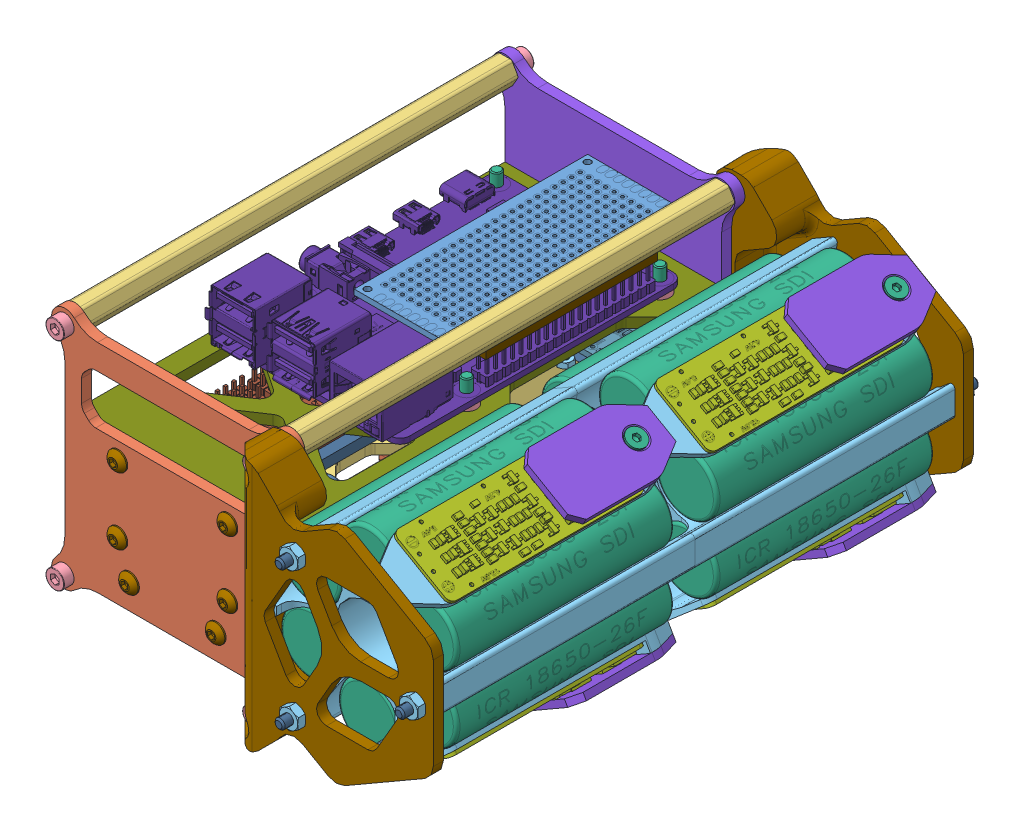
SolidWorks assembly ASM-BOX, configuration По умолчанию. Lengths in mm.
Overall size (158.14 100 172.8).
228 component instances, 28 part files, 86 mates.
Components (placement in the parent):
- ASM-level-power-1: ASM-level-power [По умолчанию] at origin size (55 22.5 129)
  - Matek Power Hub-2: Matek Power Hub [По умолчанию] at (0.0123 -25.5 35.1623) x (0 0 -1) z (1 0 0) size (36.25 3.92 36.25)
  - ACS712.step-1: ACS712.step [По умолчанию] at (17.5 -32.5 34.245) x (0 0 1) z (1 0 0) size (31.19 12.78 13.3)
  - ACS712.step-2: ACS712.step [По умолчанию] at (0 -32.5 34.245) x (0 0 1) z (1 0 0) size (31.19 12.78 13.3)
  - ACS712.step-3: ACS712.step [По умолчанию] at (-17.5 -32.5 34.245) x (0 0 1) z (1 0 0) size (31.19 12.78 13.3)
  - level-0-1: level-0 [По умолчанию] at (0 -30.5 65.5) x (1 0 0) z (0 1 0) size (55 129 7)
  - Matek Power Hub-4: Matek Power Hub [По умолчанию] at (0.0123 -25.5 95.8623) size (36.25 3.92 36.25)
  - ACS712.step-7: ACS712.step [По умолчанию] at (17.5 -32.5 96.755) x (0 0 -1) z (-1 0 0) size (31.19 12.78 13.3)
  - ACS712.step-8: ACS712.step [По умолчанию] at (0 -32.5 96.755) x (0 0 -1) z (-1 0 0) size (31.19 12.78 13.3)
  - ACS712.step-9: ACS712.step [По умолчанию] at (-17.5 -32.5 96.755) x (0 0 -1) z (-1 0 0) size (31.19 12.78 13.3)
  - 3-6-3-1: 3-6-3 [По умолчанию] at (15.35 -27.5 111.2) x (0.999975 0 -0.007062) z (0 1 0) size (6 6 2)
  - 3-6-3-2: 3-6-3 [По умолчанию] at (-15.35 -27.5 111.2) x (0.992437 0 -0.122755) z (0 1 0) size (6 6 2)
  - 3-6-3-3: 3-6-3 [По умолчанию] at (15.35 -27.5 80.5) x (0.931904 0 -0.362706) z (0 1 0) size (6 6 2)
  - 3-6-3-4: 3-6-3 [По умолчанию] at (-15.35 -27.5 80.5) x (1 0 0) z (0 1 0) size (6 6 2)
  - hex nut style 1 gradeab_iso-1: hex nut style 1 gradeab_iso [ISO - 4032 - M3 - D - N] at (15.3745 -21.9 80.5) x (1 0 0) z (0 1 0) size (5.5 6.35 2.4)
  - hex nut style 1 gradeab_iso-2: hex nut style 1 gradeab_iso [ISO - 4032 - M3 - D - N] at (-15.35 -21.9 80.5) x (1 0 0) z (0 1 0) size (5.5 6.35 2.4)
  - hex nut style 1 gradeab_iso-3: hex nut style 1 gradeab_iso [ISO - 4032 - M3 - D - N] at (15.3745 -21.9 111.2245) x (1 0 0) z (0 1 0) size (5.5 6.35 2.4)
  - hex nut style 1 gradeab_iso-4: hex nut style 1 gradeab_iso [ISO - 4032 - M3 - D - N] at (-15.35 -21.9 111.2245) x (1 0 0) z (0 1 0) size (5.5 6.35 2.4)
  - hex nut style 1 gradeab_iso-5: hex nut style 1 gradeab_iso [ISO - 4032 - M3 - D - N] at (15.3745 -21.9 50.5245) x (1 0 0) z (0 1 0) size (5.5 6.35 2.4)
  - hex nut style 1 gradeab_iso-6: hex nut style 1 gradeab_iso [ISO - 4032 - M3 - D - N] at (-15.35 -21.9 50.5245) x (1 0 0) z (0 1 0) size (5.5 6.35 2.4)
  - hex nut style 1 gradeab_iso-7: hex nut style 1 gradeab_iso [ISO - 4032 - M3 - D - N] at (15.3745 -21.9 19.8) x (1 0 0) z (0 1 0) size (5.5 6.35 2.4)
  - hex nut style 1 gradeab_iso-8: hex nut style 1 gradeab_iso [ISO - 4032 - M3 - D - N] at (-15.35 -21.9 19.8) x (1 0 0) z (0 1 0) size (5.5 6.35 2.4)
  - socket countersunk head screw_iso-1: socket countersunk head screw_iso [ISO 10642 - M3 x 8 - 8N] at (15.35 -30.11 111.2) x (0 1 0) z (-0.074206 0 0.997243) size (8 5.54 5.54)
  - socket countersunk head screw_iso-2: socket countersunk head screw_iso [ISO 10642 - M3 x 8 - 8N] at (15.35 -30.11 80.5) x (0 1 0) z (-0.12314 0 0.992389) size (8 5.54 5.54)
  - socket countersunk head screw_iso-3: socket countersunk head screw_iso [ISO 10642 - M3 x 8 - 8N] at (-15.35 -30.11 80.5) x (0 1 0) z (-0.109262 0 0.994013) size (8 5.54 5.54)
  - socket countersunk head screw_iso-4: socket countersunk head screw_iso [ISO 10642 - M3 x 8 - 8N] at (-15.35 -30.11 111.2) x (0 1 0) z (-0.069269 0 0.997598) size (8 5.54 5.54)
  - socket countersunk head screw_iso-5: socket countersunk head screw_iso [ISO 10642 - M3 x 8 - 8N] at (-22.5 -27.89 95.85) x (0 -1 0) z (-0.066693 0 0.997774) size (8 5.54 5.54)
  - socket countersunk head screw_iso-6: socket countersunk head screw_iso [ISO 10642 - M3 x 8 - 8N] at (-12.5 -27.89 95.85) x (0 -1 0) z (-0.00561 0 0.999984) size (8 5.54 5.54)
  - socket countersunk head screw_iso-7: socket countersunk head screw_iso [ISO 10642 - M3 x 8 - 8N] at (-5 -27.89 95.85) x (0 -1 0) z (0.004518 0 0.99999) size (8 5.54 5.54)
  - socket countersunk head screw_iso-8: socket countersunk head screw_iso [ISO 10642 - M3 x 8 - 8N] at (5 -27.89 95.85) x (0 -1 0) z (0.047845 0 0.998855) size (8 5.54 5.54)
  - socket countersunk head screw_iso-9: socket countersunk head screw_iso [ISO 10642 - M3 x 8 - 8N] at (12.5 -27.89 95.85) x (0 -1 0) z (0.031705 0 0.999497) size (8 5.54 5.54)
  - socket countersunk head screw_iso-10: socket countersunk head screw_iso [ISO 10642 - M3 x 8 - 8N] at (22.5 -27.89 95.85) x (0 -1 0) z (0.037692 0 0.999289) size (8 5.54 5.54)
  - hex nut style 1 gradeab_iso-13: hex nut style 1 gradeab_iso [ISO - 4032 - M3 - D - N] at (22.5 -36.48 95.85) x (1 0 0) z (0 -1 0) size (5.5 6.35 2.4)
  - hex nut style 1 gradeab_iso-14: hex nut style 1 gradeab_iso [ISO - 4032 - M3 - D - N] at (12.5 -36.48 95.85) x (1 0 0) z (0 -1 0) size (5.5 6.35 2.4)
  - hex nut style 1 gradeab_iso-15: hex nut style 1 gradeab_iso [ISO - 4032 - M3 - D - N] at (5 -36.48 95.85) x (1 0 0) z (0 -1 0) size (5.5 6.35 2.4)
  - hex nut style 1 gradeab_iso-16: hex nut style 1 gradeab_iso [ISO - 4032 - M3 - D - N] at (-5 -36.48 95.85) x (1 0 0) z (0 -1 0) size (5.5 6.35 2.4)
  - hex nut style 1 gradeab_iso-17: hex nut style 1 gradeab_iso [ISO - 4032 - M3 - D - N] at (-12.5 -36.48 95.85) x (1 0 0) z (0 -1 0) size (5.5 6.35 2.4)
  - hex nut style 1 gradeab_iso-18: hex nut style 1 gradeab_iso [ISO - 4032 - M3 - D - N] at (-22.5 -36.48 95.85) x (1 0 0) z (0 -1 0) size (5.5 6.35 2.4)
  - 3-6-3-5: 3-6-3 [По умолчанию] at (22.5 -32.5 95.85) x (1 0 0) z (0 1 0) size (6 6 2)
  - 3-6-3-6: 3-6-3 [По умолчанию] at (12.5 -32.5 95.85) x (1 0 0) z (0 1 0) size (6 6 2)
  - 3-6-3-7: 3-6-3 [По умолчанию] at (5 -32.5 95.85) x (1 0 0) z (0 1 0) size (6 6 2)
  - 3-6-3-8: 3-6-3 [По умолчанию] at (-5 -32.5 95.85) x (1 0 0) z (0 1 0) size (6 6 2)
  - 3-6-3-9: 3-6-3 [По умолчанию] at (-12.5 -32.5 95.85) x (1 0 0) z (0 1 0) size (6 6 2)
  - 3-6-3-10: 3-6-3 [По умолчанию] at (-22.5 -32.5 95.85) x (1 0 0) z (0 1 0) size (6 6 2)
  - 3-6-3-11: 3-6-3 [По умолчанию] at (-22.5 -30.5 35.15) x (1 0 0) z (0 -1 0) size (6 6 2)
  - hex nut style 1 gradeab_iso-19: hex nut style 1 gradeab_iso [ISO - 4032 - M3 - D - N] at (-22.5 -34.08 35.15) x (1 0 0) z (0 1 0) size (5.5 6.35 2.4)
  - hex nut style 1 gradeab_iso-20: hex nut style 1 gradeab_iso [ISO - 4032 - M3 - D - N] at (-12.5 -34.08 35.15) x (1 0 0) z (0 1 0) size (5.5 6.35 2.4)
  - 3-6-3-12: 3-6-3 [По умолчанию] at (-12.5 -30.5 35.15) x (1 0 0) z (0 -1 0) size (6 6 2)
  - hex nut style 1 gradeab_iso-21: hex nut style 1 gradeab_iso [ISO - 4032 - M3 - D - N] at (-5 -34.08 35.15) x (1 0 0) z (0 1 0) size (5.5 6.35 2.4)
  - hex nut style 1 gradeab_iso-22: hex nut style 1 gradeab_iso [ISO - 4032 - M3 - D - N] at (5 -34.08 35.15) x (1 0 0) z (0 1 0) size (5.5 6.35 2.4)
  - hex nut style 1 gradeab_iso-23: hex nut style 1 gradeab_iso [ISO - 4032 - M3 - D - N] at (12.5 -34.08 35.15) x (1 0 0) z (0 1 0) size (5.5 6.35 2.4)
  - hex nut style 1 gradeab_iso-24: hex nut style 1 gradeab_iso [ISO - 4032 - M3 - D - N] at (22.5 -34.08 35.15) x (1 0 0) z (0 1 0) size (5.5 6.35 2.4)
  - socket countersunk head screw_iso-11: socket countersunk head screw_iso [ISO 10642 - M3 x 8 - 8N] at (22.5 -27.89 35.15) x (0 -1 0) z (-0.037692 0 0.999289) size (8 5.54 5.54)
  - socket countersunk head screw_iso-12: socket countersunk head screw_iso [ISO 10642 - M3 x 8 - 8N] at (12.5 -27.89 35.15) x (0 -1 0) z (-0.031705 0 0.999497) size (8 5.54 5.54)
  - socket countersunk head screw_iso-13: socket countersunk head screw_iso [ISO 10642 - M3 x 8 - 8N] at (5 -27.89 35.15) x (0 -1 0) z (-0.047845 0 0.998855) size (8 5.54 5.54)
  - socket countersunk head screw_iso-14: socket countersunk head screw_iso [ISO 10642 - M3 x 8 - 8N] at (-5 -27.89 35.15) x (0 -1 0) z (-0.004518 0 0.99999) size (8 5.54 5.54)
  - socket countersunk head screw_iso-15: socket countersunk head screw_iso [ISO 10642 - M3 x 8 - 8N] at (-12.5 -27.89 35.15) x (0 -1 0) z (0.00561 0 0.999984) size (8 5.54 5.54)
  - socket countersunk head screw_iso-16: socket countersunk head screw_iso [ISO 10642 - M3 x 8 - 8N] at (-22.5 -27.89 35.15) x (0 -1 0) z (0.066693 0 0.997774) size (8 5.54 5.54)
  - 3-6-3-13: 3-6-3 [По умолчанию] at (-5 -30.5 35.15) x (1 0 0) z (0 -1 0) size (6 6 2)
  - 3-6-3-14: 3-6-3 [По умолчанию] at (5 -30.5 35.15) x (1 0 0) z (0 -1 0) size (6 6 2)
  - 3-6-3-15: 3-6-3 [По умолчанию] at (12.5 -30.5 35.15) x (1 0 0) z (0 -1 0) size (6 6 2)
  - 3-6-3-16: 3-6-3 [По умолчанию] at (22.5 -30.5 35.15) x (1 0 0) z (0 -1 0) size (6 6 2)
  - socket countersunk head screw_iso-17: socket countersunk head screw_iso [ISO 10642 - M3 x 8 - 8N] at (-15.35 -30.11 19.8) x (0 1 0) z (0.069269 0 0.997598) size (8 5.54 5.54)
  - socket countersunk head screw_iso-18: socket countersunk head screw_iso [ISO 10642 - M3 x 8 - 8N] at (15.35 -30.11 19.8) x (0 1 0) z (0.074206 0 0.997243) size (8 5.54 5.54)
  - socket countersunk head screw_iso-19: socket countersunk head screw_iso [ISO 10642 - M3 x 8 - 8N] at (-15.35 -30.11 50.5) x (0 1 0) z (0.109262 0 0.994013) size (8 5.54 5.54)
  - socket countersunk head screw_iso-20: socket countersunk head screw_iso [ISO 10642 - M3 x 8 - 8N] at (15.35 -30.11 50.5) x (0 1 0) z (0.12314 0 0.992389) size (8 5.54 5.54)
  - 3-6-3-17: 3-6-3 [По умолчанию] at (-15.35 -25.5 50.5) x (1 0 0) z (0 -1 0) size (6 6 2)
  - 3-6-3-18: 3-6-3 [По умолчанию] at (-15.35 -25.5 19.8) x (0.992437 0 0.122755) z (0 -1 0) size (6 6 2)
  - 3-6-3-19: 3-6-3 [По умолчанию] at (15.35 -25.5 50.5) x (0.931904 0 0.362706) z (0 -1 0) size (6 6 2)
  - 3-6-3-20: 3-6-3 [По умолчанию] at (15.35 -25.5 19.8) x (0.999975 0 0.007062) z (0 -1 0) size (6 6 2)
  - M3 insert nut.step-1: M3 insert nut.step [По умолчанию] at (-13 -27 4.1) size (4.49 4.48 6.21)
  - M3 insert nut.step-2: M3 insert nut.step [По умолчанию] at (13 -27 4.1) size (4.49 4.48 6.21)
  - M3 insert nut.step-3: M3 insert nut.step [По умолчанию] at (-13 -27 126.8999) size (4.49 4.48 6.21)
  - M3 insert nut.step-4: M3 insert nut.step [По умолчанию] at (13 -27 126.8999) size (4.49 4.48 6.21)
- 65-65-3-1: 65-65-3 [По умолчанию] at (0 -2 -2) size (100 100 3)
- socket button head screw_iso-1: socket button head screw_iso [ISO 7380 - M3 x 8 - 8N] at (13 -27 -3.65) x (0 0 1) z (-1 0 0) size (9.65 5.7 5.7)
- socket button head screw_iso-2: socket button head screw_iso [ISO 7380 - M3 x 8 - 8N] at (-13 -27 -3.65) x (0 0 1) z (-1 0 0) size (9.65 5.7 5.7)
- asm-level-pwn-1: asm-level-pwn [По умолчанию] at (0 -16.5 65.5) x (1 0 0) z (0 1 0) size (65 129.01 16.99)
  - level-1-2: level-1 [По умолчанию] at origin size (65 129 7.45)
  - 3-6-3-33: 3-6-3 [По умолчанию] at (-25.8 -59.9 3) size (6 6 2)
  - 3-6-3-34: 3-6-3 [По умолчанию] at (-7 -59.9 3) size (6 6 2)
  - 3-6-3-35: 3-6-3 [По умолчанию] at (-25.8 -4 3) x (0.841268 -0.540619 0) z (0 0 1) size (6 6 2)
  - 3-6-3-36: 3-6-3 [По умолчанию] at (-7 -4 3) size (6 6 2)
  - 3-6-3-37: 3-6-3 [По умолчанию] at (-25.8 4 3) size (6 6 2)
  - 3-6-3-38: 3-6-3 [По умолчанию] at (-7 4 3) size (6 6 2)
  - 3-6-3-39: 3-6-3 [По умолчанию] at (-25.8 59.9 3) size (6 6 2)
  - 3-6-3-40: 3-6-3 [По умолчанию] at (-7 59.9 3) size (6 6 2)
  - socket countersunk head screw_iso-33: socket countersunk head screw_iso [ISO 10642 - M3 x 10 - 10N] at (-7 -4 0.39) x (0 0 1) z (-0.999892 0.014671 0) size (10 5.54 5.54)
  - socket countersunk head screw_iso-34: socket countersunk head screw_iso [ISO 10642 - M3 x 10 - 10N] at (-7 59.9 0.39) x (0 0 1) z (-0.999933 0.011601 0) size (10 5.54 5.54)
  - socket countersunk head screw_iso-35: socket countersunk head screw_iso [ISO 10642 - M3 x 10 - 10N] at (-25.8 59.9 0.39) x (0 0 1) z (-0.999806 0.019696 0) size (10 5.54 5.54)
  - socket countersunk head screw_iso-36: socket countersunk head screw_iso [ISO 10642 - M3 x 10 - 10N] at (-25.8 4 0.39) x (0 0 1) z (-0.999874 0.015878 0) size (10 5.54 5.54)
  - socket countersunk head screw_iso-37: socket countersunk head screw_iso [ISO 10642 - M3 x 10 - 10N] at (-25.8 -4 0.39) x (0 0 1) z (-0.999899 0.014235 0) size (10 5.54 5.54)
  - socket countersunk head screw_iso-38: socket countersunk head screw_iso [ISO 10642 - M3 x 10 - 10N] at (-7 4 0.39) x (0 0 1) z (-0.999995 0.003285 0) size (10 5.54 5.54)
  - socket countersunk head screw_iso-39: socket countersunk head screw_iso [ISO 10642 - M3 x 10 - 10N] at (-7 -59.9 0.39) x (0 0 1) z (-0.999968 0.008038 0) size (10 5.54 5.54)
  - socket countersunk head screw_iso-40: socket countersunk head screw_iso [ISO 10642 - M3 x 10 - 10N] at (-25.8 -59.9 0.39) x (0 0 1) z (-0.999943 0.010711 0) size (10 5.54 5.54)
  - 12Channel PWM-5: 12Channel PWM [Default] at (-16.4 31.95 5) x (1 0 0) z (0 -1 0) size (25.4 7.55 62.5)
  - 12Channel PWM-6: 12Channel PWM [Default] at (-16.4 -31.95 5) x (1 0 0) z (0 -1 0) size (25.4 7.55 62.5)
  - 20-80-shild-2: 20-80-shild [По умолчанию] at (20 0 5) x (0 -1 0) z (0 0 1) size (80 20 1.6)
  - 2-5-2-1: 2-5-2 [По умолчанию] at (12.5 -37.5 3) size (5 5 2)
  - 2-5-2-2: 2-5-2 [По умолчанию] at (27.5 -37.5 3) x (0.979435 -0.201761 0) z (0 0 1) size (5 5 2)
  - 2-5-2-3: 2-5-2 [По умолчанию] at (12.5 37.5 3) size (5 5 2)
  - 2-5-2-4: 2-5-2 [По умолчанию] at (27.5 37.5 3) size (5 5 2)
  - 16Bit I2C ADC+PGA - ADS1115-3: 16Bit I2C ADC+PGA - ADS1115 [По умолчанию] at (16.07 -52.658 5) x (-1 0 0) z (0 0 1) size (27.94 17.27 2.74)
  - 16Bit I2C ADC+PGA - ADS1115-4: 16Bit I2C ADC+PGA - ADS1115 [По умолчанию] at (16.07 52.658 5) size (27.94 17.27 2.74)
  - 3-6-3-41: 3-6-3 [По умолчанию] at (27.5 58.5 3) x (0.99991 0.013401 0) z (0 0 1) size (6 6 2)
  - 3-6-3-42: 3-6-3 [По умолчанию] at (4.64 58.5 3) size (6 6 2)
  - 3-6-3-43: 3-6-3 [По умолчанию] at (4.64 -58.5 3) x (0.998248 0.059171 0) z (0 0 1) size (6 6 2)
  - 3-6-3-44: 3-6-3 [По умолчанию] at (27.5 -58.5 3) x (0.961366 -0.275274 0) z (0 0 1) size (6 6 2)
  - socket countersunk head screw_iso-41: socket countersunk head screw_iso [ISO 10642 - M3 x 10 - 10N] at (27.5 58.5 0.265) x (0 0 1) z (-0.999931 -0.011786 0) size (10 5.54 5.54)
  - socket countersunk head screw_iso-42: socket countersunk head screw_iso [ISO 10642 - M3 x 10 - 10N] at (4.64 58.5 0.265) x (0 0 1) z (-0.999999 0.001606 0) size (10 5.54 5.54)
  - socket countersunk head screw_iso-43: socket countersunk head screw_iso [ISO 10642 - M3 x 10 - 10N] at (4.64 -58.5 0.265) x (0 0 1) z (-0.999998 -0.001805 0) size (10 5.54 5.54)
  - socket countersunk head screw_iso-44: socket countersunk head screw_iso [ISO 10642 - M3 x 10 - 10N] at (27.5 -58.5 0.265) x (0 0 1) z (-0.999975 -0.007128 0) size (10 5.54 5.54)
  - countersunk flat head cross recess screw_iso-1: countersunk flat head cross recess screw_iso [ISO 7046-1 - M2 x 8 - Z - 8N] at (27.5 -37.5 0.3) x (0 0 1) z (-0.99999 -0.004571 0) size (8 3.8 3.8)
  - countersunk flat head cross recess screw_iso-2: countersunk flat head cross recess screw_iso [ISO 7046-1 - M2 x 8 - Z - 8N] at (12.5 -37.5 0.3) x (0 0 1) z (-0.999692 0.024831 0) size (8 3.8 3.8)
  - countersunk flat head cross recess screw_iso-3: countersunk flat head cross recess screw_iso [ISO 7046-1 - M2 x 8 - Z - 8N] at (27.5 37.5 0.3) x (0 0 1) z (-0.999277 0.038023 0) size (8 3.8 3.8)
  - countersunk flat head cross recess screw_iso-4: countersunk flat head cross recess screw_iso [ISO 7046-1 - M2 x 8 - Z - 8N] at (12.5 37.5 0.3) x (0 0 1) z (-0.999541 0.030296 0) size (8 3.8 3.8)
  - hex nut style 1 gradeab_iso-38: hex nut style 1 gradeab_iso [ISO - 4032 - M3 - D - N] at (4.64 -58.5 9.0002) size (5.5 6.35 2.4)
  - hex nut style 1 gradeab_iso-39: hex nut style 1 gradeab_iso [ISO - 4032 - M3 - D - N] at (27.5 -58.5 9.0002) size (5.5 6.35 2.4)
  - hex nut style 1 gradeab_iso-41: hex nut style 1 gradeab_iso [ISO - 4032 - M3 - D - N] at (-25.8 -59.9 8.91) size (5.5 6.35 2.4)
  - hex nut style 1 gradeab_iso-42: hex nut style 1 gradeab_iso [ISO - 4032 - M3 - D - N] at (-7 4 8.91) size (5.5 6.35 2.4)
  - hex nut style 1 gradeab_iso-43: hex nut style 1 gradeab_iso [ISO - 4032 - M3 - D - N] at (-7 -4 8.9) size (5.5 6.35 2.4)
  - hex nut style 1 gradeab_iso-44: hex nut style 1 gradeab_iso [ISO - 4032 - M3 - D - N] at (-25.8 4 8.91) size (5.5 6.35 2.4)
  - hex nut style 1 gradeab_iso-45: hex nut style 1 gradeab_iso [ISO - 4032 - M3 - D - N] at (-25.8 -4 8.91) size (5.5 6.35 2.4)
  - hex nut style 1 gradeab_iso-46: hex nut style 1 gradeab_iso [ISO - 4032 - M3 - D - N] at (-25.8 59.9 8.91) size (5.5 6.35 2.4)
  - hex nut style 1 gradeab_iso-47: hex nut style 1 gradeab_iso [ISO - 4032 - M3 - D - N] at (-7 59.9 8.9) size (5.5 6.35 2.4)
  - hex nut style 1 gradeab_iso-48: hex nut style 1 gradeab_iso [ISO - 4032 - M3 - D - N] at (4.64 58.5 9.0002) size (5.5 6.35 2.4)
  - hex nut style 1 gradeab_iso-50: hex nut style 1 gradeab_iso [ISO - 4032 - M3 - D - N] at (-7 -59.9 8.91) size (5.5 6.35 2.4)
  - hex nut style 1 gradeab_iso-51: hex nut style 1 gradeab_iso [ISO - 4032 - M3 - D - N] at (27.5 58.5 9.0002) size (5.5 6.35 2.4)
  - hex nut style 1 gradeab_iso-52: hex nut style 1 gradeab_iso [ISO - 4032 - M2 - D - N] at (12.5 -37.5 8.2) size (4 4.62 1.6)
  - hex nut style 1 gradeab_iso-53: hex nut style 1 gradeab_iso [ISO - 4032 - M2 - D - N] at (27.5 -37.5 8.2) size (4 4.62 1.6)
  - hex nut style 1 gradeab_iso-54: hex nut style 1 gradeab_iso [ISO - 4032 - M2 - D - N] at (12.5 37.5 8.2) size (4 4.62 1.6)
  - hex nut style 1 gradeab_iso-55: hex nut style 1 gradeab_iso [ISO - 4032 - M2 - D - N] at (27.5 37.5 8.2) size (4 4.62 1.6)
  - M3 insert nut.step-1: M3 insert nut.step [По умолчанию] at (-16.5 61.4 -0.5) x (1 0 0) z (0 1 0) size (4.49 4.48 6.21)
  - M3 insert nut.step-2: M3 insert nut.step [По умолчанию] at (16.5 61.4 -0.5) x (1 0 0) z (0 1 0) size (4.49 4.48 6.21)
  - M3 insert nut.step-3: M3 insert nut.step [По умолчанию] at (16.5 -61.4001 -0.5) x (1 0 0) z (0 1 0) size (4.49 4.48 6.21)
  - M3 insert nut.step-4: M3 insert nut.step [По умолчанию] at (-16.5 -61.4001 -0.5) x (1 0 0) z (0 1 0) size (4.49 4.48 6.21)
- ASM-level-raspberry-pi-1: ASM-level-raspberry-pi [По умолчанию] at (0 3.5 65.5) x (-1 0 0) z (0 1 0) size (65 129.01 28.74)
  - level-2-1: level-2 [По умолчанию] at origin size (65 129 7)
  - Raspberry Pi 4 Model B-1: Raspberry Pi 4 Model B [По умолчанию] at (0 -15 5.79) x (0 1 0) z (1 0 0) size (88.99 19.91 58.4)
  - 3-6-3-1: 3-6-3 [По умолчанию] at (-24.5 -54 3) size (6 6 2)
  - 3-6-3-2: 3-6-3 [По умолчанию] at (-24.5 4 3) size (6 6 2)
  - 3-6-3-3: 3-6-3 [По умолчанию] at (24.5 4 3) size (6 6 2)
  - 3-6-3-4: 3-6-3 [По умолчанию] at (24.5 -54 3) x (0.98212 -0.188257 0) z (0 0 1) size (6 6 2)
  - socket countersunk head screw_iso-1: socket countersunk head screw_iso [ISO 10642 - M3 x 10 - 10N] at (24.5 -54 0.39) x (0 0 1) z (-0.999977 -0.006797 0) size (10 5.54 5.54)
  - socket countersunk head screw_iso-2: socket countersunk head screw_iso [ISO 10642 - M3 x 10 - 10N] at (24.5 4 0.39) x (0 0 1) z (-0.999917 -0.012873 0) size (10 5.54 5.54)
  - socket countersunk head screw_iso-3: socket countersunk head screw_iso [ISO 10642 - M3 x 10 - 10N] at (-24.5 4 0.39) x (0 0 1) z (-0.999928 -0.012001 0) size (10 5.54 5.54)
  - socket countersunk head screw_iso-4: socket countersunk head screw_iso [ISO 10642 - M3 x 10 - 10N] at (-24.5 -54 0.39) x (0 0 1) z (-1 -0.000767 0) size (10 5.54 5.54)
  - ASM-shild-raspberry-1: ASM-shild-raspberry [По умолчанию] at (-22.18 0.88 25.14) x (1 0 0) z (0 1 0) size (30 10.65 70)
    - 40 pin connector header smt v3.step-1: 40 pin connector header smt v3.step [По умолчанию] at origin size (5.18 10.05 51.4)
    - Breadboard 30 х 70 mm.step-1: Breadboard 30 х 70 mm.step [По умолчанию] at (7.5097 0.4 -23.0097) size (30 1.65 70)
  - M3 insert nut.step-1: M3 insert nut.step [По умолчанию] at (16.5 -61.4 -0.5) x (1 0 0) z (0 -1 0) size (4.49 4.48 6.21)
  - M3 insert nut.step-2: M3 insert nut.step [По умолчанию] at (-16.5 -61.4 -0.5) x (1 0 0) z (0 -1 0) size (4.49 4.48 6.21)
  - M3 insert nut.step-3: M3 insert nut.step [По умолчанию] at (16.5 61.4001 -0.5) x (1 0 0) z (0 -1 0) size (4.49 4.48 6.21)
  - M3 insert nut.step-4: M3 insert nut.step [По умолчанию] at (-16.5 61.4001 -0.5) x (1 0 0) z (0 -1 0) size (4.49 4.48 6.21)
- socket button head screw_iso-3: socket button head screw_iso [ISO 7380 - M3 x 8 - 8N] at (-16.5 -17 -3.65) x (0 0 1) z (-1 0 0) size (9.65 5.7 5.7)
- socket button head screw_iso-4: socket button head screw_iso [ISO 7380 - M3 x 8 - 8N] at (16.5 -17 -3.65) x (0 0 1) z (-1 0 0) size (9.65 5.7 5.7)
- socket button head screw_iso-5: socket button head screw_iso [ISO 7380 - M3 x 8 - 8N] at (16.5 3 -3.65) x (0 0 1) z (-1 0 0) size (9.65 5.7 5.7)
- socket button head screw_iso-6: socket button head screw_iso [ISO 7380 - M3 x 8 - 8N] at (-16.5 3 -3.65) x (0 0 1) z (-1 0 0) size (9.65 5.7 5.7)
- 65-65-3-down-1: 65-65-3-down [По умолчанию] at (0 -2 130) size (100 100 3)
- socket button head screw_iso-7: socket button head screw_iso [ISO 7380 - M3 x 8 - 8N] at (16.5 3 134.65) x (0 0 -1) z (1 0 0) size (9.65 5.7 5.7)
- socket button head screw_iso-8: socket button head screw_iso [ISO 7380 - M3 x 8 - 8N] at (-16.5 3 134.65) x (0 0 -1) z (1 0 0) size (9.65 5.7 5.7)
- socket button head screw_iso-9: socket button head screw_iso [ISO 7380 - M3 x 8 - 8N] at (-16.5 -17 134.65) x (0 0 -1) z (1 0 0) size (9.65 5.7 5.7)
- socket button head screw_iso-11: socket button head screw_iso [ISO 7380 - M3 x 8 - 8N] at (16.5 -17 134.65) x (0 0 -1) z (1 0 0) size (9.65 5.7 5.7)
- socket button head screw_iso-12: socket button head screw_iso [ISO 7380 - M3 x 8 - 8N] at (13 -27 134.65) x (0 0 -1) z (1 0 0) size (9.65 5.7 5.7)
- socket button head screw_iso-13: socket button head screw_iso [ISO 7380 - M3 x 8 - 8N] at (-13 -27 134.65) x (0 0 -1) z (1 0 0) size (9.65 5.7 5.7)
- stoyka-7-129-1: stoyka-7-129 [По умолчанию] at (-32.5 30.5 1) size (7.77 7 129)
- M3 insert nut.step-1: M3 insert nut.step [По умолчанию] at (-32.5 30.5 126.9) size (4.49 4.48 6.21)
- M3 insert nut.step-2: M3 insert nut.step [По умолчанию] at (-32.5 30.5 4.1) size (4.49 4.48 6.21)
- M3 insert nut.step-3: M3 insert nut.step [По умолчанию] at (-32.5 -34.5 4.1) size (4.49 4.48 6.21)
- M3 insert nut.step-4: M3 insert nut.step [По умолчанию] at (32.5 30.5 4.1) size (4.49 4.48 6.21)
- M3 insert nut.step-5: M3 insert nut.step [По умолчанию] at (32.5 -34.5 4.1) size (4.49 4.48 6.21)
- M3 insert nut.step-6: M3 insert nut.step [По умолчанию] at (-32.5 -34.5 126.9) size (4.49 4.48 6.21)
- M3 insert nut.step-7: M3 insert nut.step [По умолчанию] at (32.5 30.5 126.9) size (4.49 4.48 6.21)
- M3 insert nut.step-8: M3 insert nut.step [По умолчанию] at (32.5 -34.5 126.9) size (4.49 4.48 6.21)
- stoyka-7-129-2: stoyka-7-129 [По умолчанию] at (-32.5 -34.5 1) size (7.77 7 129)
- stoyka-7-129-3: stoyka-7-129 [По умолчанию] at (32.5 30.5 1) size (7.77 7 129)
- stoyka-7-129-4: stoyka-7-129 [По умолчанию] at (32.5 -34.5 1) size (7.77 7 129)
- socket head cap screw_iso-3: socket head cap screw_iso [ISO 4762 M3 x 8 - 8N] at (-32.5 30.5 -5) x (0 0 1) z (-1 0 0) size (11 5.5 5.5)
- socket head cap screw_iso-4: socket head cap screw_iso [ISO 4762 M3 x 8 - 8N] at (-32.5 -34.5 -5) x (0 0 1) z (-1 0 0) size (11 5.5 5.5)
- socket head cap screw_iso-7: socket head cap screw_iso [ISO 4762 M3 x 8 - 8N] at (-32.5 -34.5 136) x (0 0 -1) z (1 0 0) size (11 5.5 5.5)
- socket head cap screw_iso-8: socket head cap screw_iso [ISO 4762 M3 x 8 - 8N] at (-32.5 30.5 136) x (0 0 -1) z (1 0 0) size (11 5.5 5.5)
- ASM_battery_18650-1: ASM_battery_18650 [По умолчанию] at (62.5 -2 -12.5) x (0.866025 -0.5 0) z (0 0 1) size (65.8 63.25 78)
  - gerjatel_18650-1: gerjatel_18650 [По умолчанию] at origin size (56.64 57.5 78)
  - Samsung icr18650-1: Samsung icr18650 [Predeterminado] at (-10 17.3205 6.5) x (0.574262 0.818672 0) z (0 0 1) size (18.4 18.4 65)
  - Samsung icr18650-2: Samsung icr18650 [Predeterminado] at (10 17.3205 6.5) x (0.996121 -0.08799 0) z (0 0 1) size (18.4 18.4 65)
  - Samsung icr18650-3: Samsung icr18650 [Predeterminado] at (20 0 6.5) x (0.421859 -0.906661 0) z (0 0 1) size (18.4 18.4 65)
  - Samsung icr18650-4: Samsung icr18650 [Predeterminado] at (10 -17.3205 6.5) x (-0.574262 -0.818672 0) z (0 0 1) size (18.4 18.4 65)
  - Samsung icr18650-5: Samsung icr18650 [Predeterminado] at (-10 -17.3205 6.5) x (-0.996121 0.08799 0) z (0 0 1) size (18.4 18.4 65)
  - Samsung icr18650-6: Samsung icr18650 [Predeterminado] at (-20 0 6.5) x (-0.421859 0.906661 0) z (0 0 1) size (18.4 18.4 65)
  - Battery Protection - 3S-20A.stp-1: Battery Protection - 3S-20A.stp [По умолчанию] at (0.033 28 40.5275) x (0 0 1) z (0 1 0) size (59.06 20.07 3.17)
  - Battery Protection - 3S-20A.stp-2: Battery Protection - 3S-20A.stp [По умолчанию] at (24.2322 -14.0286 40.5275) x (0 0 1) z (0.866025 -0.5 0) size (59.06 20.07 3.17)
  - M3 insert nut.step-1: M3 insert nut.step [По умолчанию] at (24.1621 -13.95 7.5) x (0.459729 0.796273 -0.39319) z (0.866025 -0.5 0) size (4.49 4.48 6.21)
  - M3 insert nut.step-2: M3 insert nut.step [По умолчанию] at (0 27.9 7.5) x (-0.919457 0 -0.39319) z (0 1 0) size (4.49 4.48 6.21)
  - radiator-1: radiator [По умолчанию] at (32.4385 -5.8148 3.3587) x (0.5 0.866025 0) z (0 0 1) size (20 2 34.23)
  - socket countersunk head screw_iso-1: socket countersunk head screw_iso [ISO 10642 - M3 x 8 - 8N] at (28.6741 -16.555 7.5) x (-0.866025 0.5 0) z (0.490678 0.849879 -0.1922) size (8 5.54 5.54)
  - socket countersunk head screw_iso-2: socket countersunk head screw_iso [ISO 10642 - M3 x 8 - 8N] at (0 33.11 7.5) x (0 -1 0) z (-0.981356 0 -0.1922) size (8 5.54 5.54)
  - radiator-2: radiator [По умолчанию] at (-11.1835 31 3.3587) x (-1 0 0) z (0 0 1) size (20 2 34.23)
- ASM_battery_18650-2: ASM_battery_18650 [По умолчанию] at (62.5 -2 65.5) x (0.866025 -0.5 0) z (0 0 1) size (65.8 63.25 78)
  - gerjatel_18650-1: gerjatel_18650 [По умолчанию] at origin size (56.64 57.5 78)
  - Samsung icr18650-1: Samsung icr18650 [Predeterminado] at (-10 17.3205 6.5) x (0.574262 0.818672 0) z (0 0 1) size (18.4 18.4 65)
  - Samsung icr18650-2: Samsung icr18650 [Predeterminado] at (10 17.3205 6.5) x (0.996121 -0.08799 0) z (0 0 1) size (18.4 18.4 65)
  - Samsung icr18650-3: Samsung icr18650 [Predeterminado] at (20 0 6.5) x (0.421859 -0.906661 0) z (0 0 1) size (18.4 18.4 65)
  - Samsung icr18650-4: Samsung icr18650 [Predeterminado] at (10 -17.3205 6.5) x (-0.574262 -0.818672 0) z (0 0 1) size (18.4 18.4 65)
  - Samsung icr18650-5: Samsung icr18650 [Predeterminado] at (-10 -17.3205 6.5) x (-0.996121 0.08799 0) z (0 0 1) size (18.4 18.4 65)
  - Samsung icr18650-6: Samsung icr18650 [Predeterminado] at (-20 0 6.5) x (-0.421859 0.906661 0) z (0 0 1) size (18.4 18.4 65)
  - Battery Protection - 3S-20A.stp-1: Battery Protection - 3S-20A.stp [По умолчанию] at (0.033 28 40.5275) x (0 0 1) z (0 1 0) size (59.06 20.07 3.17)
  - Battery Protection - 3S-20A.stp-2: Battery Protection - 3S-20A.stp [По умолчанию] at (24.2322 -14.0286 40.5275) x (0 0 1) z (0.866025 -0.5 0) size (59.06 20.07 3.17)
  - M3 insert nut.step-1: M3 insert nut.step [По умолчанию] at (24.1621 -13.95 7.5) x (0.459729 0.796273 -0.39319) z (0.866025 -0.5 0) size (4.49 4.48 6.21)
  - M3 insert nut.step-2: M3 insert nut.step [По умолчанию] at (0 27.9 7.5) x (-0.919457 0 -0.39319) z (0 1 0) size (4.49 4.48 6.21)
  - radiator-1: radiator [По умолчанию] at (32.4385 -5.8148 3.3587) x (0.5 0.866025 0) z (0 0 1) size (20 2 34.23)
  - socket countersunk head screw_iso-1: socket countersunk head screw_iso [ISO 10642 - M3 x 8 - 8N] at (28.6741 -16.555 7.5) x (-0.866025 0.5 0) z (0.490678 0.849879 -0.1922) size (8 5.54 5.54)
  - socket countersunk head screw_iso-2: socket countersunk head screw_iso [ISO 10642 - M3 x 8 - 8N] at (0 33.11 7.5) x (0 -1 0) z (-0.981356 0 -0.1922) size (8 5.54 5.54)
  - radiator-2: radiator [По умолчанию] at (-11.1835 31 3.3587) x (-1 0 0) z (0 0 1) size (20 2 34.23)
- crep-battery-1: crep-battery [По умолчанию] at (62.5 -2 -15.5) x (0 1 0) z (0 0 1) size (75 64 13.5)
- crep-battery-2: crep-battery [По умолчанию] at (62.5 -2 146.5) x (0 -1 0) z (0 0 -1) size (75 64 13.5)
- socket head cap screw_iso-10: socket head cap screw_iso [ISO 4762 M3 x 12 - 12N] at (32.5 30.5 142) x (0 0 -1) z (1 0 0) size (15 5.5 5.5)
- socket head cap screw_iso-11: socket head cap screw_iso [ISO 4762 M3 x 12 - 12N] at (32.5 -34.5 142) x (0 0 -1) z (1 0 0) size (15 5.5 5.5)
- socket head cap screw_iso-12: socket head cap screw_iso [ISO 4762 M3 x 12 - 12N] at (32.5 -34.5 -11) x (0 0 1) z (-1 0 0) size (15 5.5 5.5)
- socket head cap screw_iso-13: socket head cap screw_iso [ISO 4762 M3 x 12 - 12N] at (32.5 30.5 -11) x (0 0 1) z (-1 0 0) size (15 5.5 5.5)
- hex nut style 1 gradeab_iso-1: hex nut style 1 gradeab_iso [ISO - 4032 - M3 - D - N] at (50.5 18.7846 148.9) size (5.5 6.35 2.4)
- hex nut style 1 gradeab_iso-2: hex nut style 1 gradeab_iso [ISO - 4032 - M3 - D - N] at (50.5 -22.7846 148.9) size (5.5 6.35 2.4)
- hex nut style 1 gradeab_iso-3: hex nut style 1 gradeab_iso [ISO - 4032 - M3 - D - N] at (86.5 -2 148.9) size (5.5 6.35 2.4)
- hex nut style 1 gradeab_iso-4: hex nut style 1 gradeab_iso [ISO - 4032 - M3 - D - N] at (50.5 -22.7846 -17.9) x (0.923728 0.383049 0) z (0 0 -1) size (5.5 6.35 2.4)
- hex nut style 1 gradeab_iso-5: hex nut style 1 gradeab_iso [ISO - 4032 - M3 - D - N] at (50.5 18.7846 -17.9) x (0.923728 0.383049 0) z (0 0 -1) size (5.5 6.35 2.4)
- hex nut style 1 gradeab_iso-6: hex nut style 1 gradeab_iso [ISO - 4032 - M3 - D - N] at (86.5 -2 -17.9) x (0.923728 0.383049 0) z (0 0 -1) size (5.5 6.35 2.4)
- 172.8-3-1: 172.8-3 [По умолчанию] at (50.5 -22.7846 -20.9) size (3 3 172.8)
- 172.8-3-2: 172.8-3 [По умолчанию] at (50.5 18.7846 -20.9) x (-0.5 -0.866025 0) z (0 0 1) size (3 3 172.8)
- 172.8-3-3: 172.8-3 [По умолчанию] at (86.5 -2 -20.9) x (-0.5 0.866025 0) z (0 0 1) size (3 3 172.8)
Mates (geometry in assembly coordinates):
- Концентричный1: concentric anti-aligned: cylinder of ASM-level-power-1/level-0-1 through (13 -27 7) axis (0 0 -1) radius 2; cylinder of 65-65-3-1 through (13 -27 -9) axis (0 0 1) radius 1.75
- Концентричный2: concentric anti-aligned: cylinder of ASM-level-power-1/level-0-1 through (-13 -27 7) axis (0 0 -1) radius 2; cylinder of 65-65-3-1 through (-13 -27 -9) axis (0 0 1) radius 1.75
- Концентричный3: concentric anti-aligned: cylinder of ASM-level-power-1/level-0-1 through (-13 -27 8) axis (0 0 -1) radius 3.5; cylinder of 65-65-3-1 through (-13 -27 -9) axis (0 0 1) radius 1.75
- Совпадение1: coincident anti-aligned: plane of ASM-level-power-1/level-0-1 through (0 -27.5 1) normal (0 0 -1); plane of 65-65-3-1 through (0 -2 1) normal (0 0 1)
- Концентричный4: concentric anti-aligned: cylinder of 65-65-3-1 through (13 -27 -9) axis (0 0 1) radius 1.75; cylinder of socket button head screw_iso-1 through (13 -27 -3.65) axis (0 0 -1) radius 2.85
- Совпадение2: coincident anti-aligned: plane of 65-65-3-1 through (0 -2 -2) normal (0 0 -1); plane of socket button head screw_iso-1 through (13 -25.5 -2) normal (0 0 1)
- Концентричный5: concentric anti-aligned: cylinder of 65-65-3-1 through (-13 -27 -9) axis (0 0 1) radius 1.75; cylinder of socket button head screw_iso-2 through (-13 -27 -3.65) axis (0 0 -1) radius 2.85
- Совпадение3: coincident anti-aligned: plane of 65-65-3-1 through (0 -2 -2) normal (0 0 -1); plane of socket button head screw_iso-2 through (-13 -25.5 -2) normal (0 0 1)
- Концентричный6: concentric anti-aligned: cylinder of 65-65-3-1 through (16.5 -17 -9) axis (0 0 1) radius 1.75; cylinder of asm-level-pwn-1/level-1-2 through (16.5 -17 8) axis (0 0 -1) radius 3.5
- Совпадение4: coincident anti-aligned: plane of 65-65-3-1 through (0 -2 1) normal (0 0 1); plane of asm-level-pwn-1/level-1-2 through (0 -13.5 1) normal (0 0 -1)
- Параллельность2: parallel aligned: plane of ASM-level-power-1/level-0-1 through (0 -30.5 65.5) normal (0 -1 0); plane of asm-level-pwn-1/level-1-2 through (0 -16.5 65.5) normal (0 -1 0)
- Концентричный7: concentric anti-aligned: cylinder of 65-65-3-1 through (16.5 3 -9) axis (0 0 1) radius 1.75; cylinder of ASM-level-raspberry-pi-1/level-2-1 through (16.5 3 8) axis (0 0 -1) radius 3.5
- Совпадение5: coincident anti-aligned: plane of 65-65-3-1 through (0 -2 1) normal (0 0 1); plane of ASM-level-raspberry-pi-1/level-2-1 through (0 6.5 1) normal (0 0 -1)
- Параллельность3: parallel anti-aligned: plane of asm-level-pwn-1/level-1-2 through (0 -13.5 65.5) normal (0 1 0); plane of ASM-level-raspberry-pi-1/level-2-1 through (0 3.5 65.5) normal (0 -1 0)
- Концентричный8: concentric anti-aligned: cylinder of 65-65-3-1 through (-16.5 -17 -9) axis (0 0 1) radius 1.75; cylinder of socket button head screw_iso-3 through (-16.5 -17 -3.65) axis (0 0 -1) radius 2.85
- Совпадение7: coincident anti-aligned: plane of 65-65-3-1 through (0 -2 -2) normal (0 0 -1); plane of socket button head screw_iso-3 through (-16.5 -15.5 -2) normal (0 0 1)
- Концентричный9: concentric anti-aligned: cylinder of 65-65-3-1 through (16.5 -17 -9) axis (0 0 1) radius 1.75; cylinder of socket button head screw_iso-4 through (16.5 -17 -3.65) axis (0 0 -1) radius 2.85
- Совпадение8: coincident anti-aligned: plane of 65-65-3-1 through (0 -2 -2) normal (0 0 -1); plane of socket button head screw_iso-4 through (16.5 -15.5 -2) normal (0 0 1)
- Концентричный10: concentric anti-aligned: cylinder of 65-65-3-1 through (16.5 3 -9) axis (0 0 1) radius 1.75; cylinder of socket button head screw_iso-5 through (16.5 3 -3.65) axis (0 0 -1) radius 2.85
- Совпадение9: coincident anti-aligned: plane of 65-65-3-1 through (0 -2 -2) normal (0 0 -1); plane of socket button head screw_iso-5 through (16.5 4.5 -2) normal (0 0 1)
- Концентричный11: concentric anti-aligned: cylinder of 65-65-3-1 through (-16.5 3 -9) axis (0 0 1) radius 1.75; cylinder of socket button head screw_iso-6 through (-16.5 3 -3.65) axis (0 0 -1) radius 2.85
- Совпадение10: coincident anti-aligned: plane of 65-65-3-1 through (0 -2 -2) normal (0 0 -1); plane of socket button head screw_iso-6 through (-16.5 4.5 -2) normal (0 0 1)
- Концентричный12: concentric aligned: cylinder of 65-65-3-1 through (-32.5 -34.5 1) axis (0 0 -1) radius 1.625; cylinder of 65-65-3-down-1 through (-32.5 -34.5 133) axis (0 0 -1) radius 1.625
- Концентричный13: concentric aligned: cylinder of 65-65-3-1 through (32.5 -34.5 1) axis (0 0 -1) radius 1.625; cylinder of 65-65-3-down-1 through (32.5 -34.5 133) axis (0 0 -1) radius 1.625
- Совпадение11: coincident anti-aligned: plane of ASM-level-power-1/level-0-1 through (0 -27.5 130) normal (0 0 1); plane of 65-65-3-down-1 through (0 -2 130) normal (0 0 -1)
- Концентричный14: concentric aligned: cylinder of 65-65-3-down-1 through (16.5 3 123) axis (0 0 1) radius 1.75; cylinder of socket button head screw_iso-7 through (16.5 3 134.65) axis (0 0 1) radius 2.85
- Совпадение12: coincident anti-aligned: plane of 65-65-3-down-1 through (0 -2 133) normal (0 0 1); plane of socket button head screw_iso-7 through (16.5 4.5 133) normal (0 0 -1)
- Концентричный15: concentric aligned: cylinder of 65-65-3-down-1 through (-16.5 3 123) axis (0 0 1) radius 1.75; cylinder of socket button head screw_iso-8 through (-16.5 3 134.65) axis (0 0 1) radius 2.85
- Совпадение13: coincident anti-aligned: plane of 65-65-3-down-1 through (0 -2 133) normal (0 0 1); plane of socket button head screw_iso-8 through (-16.5 4.5 133) normal (0 0 -1)
- Концентричный16: concentric aligned: cylinder of 65-65-3-down-1 through (-16.5 -17 123) axis (0 0 1) radius 1.75; cylinder of socket button head screw_iso-9 through (-16.5 -17 134.65) axis (0 0 1) radius 2.85
- Совпадение14: coincident anti-aligned: plane of 65-65-3-down-1 through (0 -2 133) normal (0 0 1); plane of socket button head screw_iso-9 through (-16.5 -15.5 133) normal (0 0 -1)
- Концентричный18: concentric aligned: cylinder of 65-65-3-down-1 through (16.5 -17 123) axis (0 0 1) radius 1.75; cylinder of socket button head screw_iso-11 through (16.5 -17 134.65) axis (0 0 1) radius 2.85
- Совпадение15: coincident anti-aligned: plane of 65-65-3-down-1 through (0 -2 133) normal (0 0 1); plane of socket button head screw_iso-11 through (16.5 -15.5 133) normal (0 0 -1)
- Концентричный19: concentric aligned: cylinder of 65-65-3-down-1 through (13 -27 123) axis (0 0 1) radius 1.75; cylinder of socket button head screw_iso-12 through (13 -27 134.65) axis (0 0 1) radius 2.85
- Совпадение16: coincident anti-aligned: plane of 65-65-3-down-1 through (0 -2 133) normal (0 0 1); plane of socket button head screw_iso-12 through (13 -25.5 133) normal (0 0 -1)
- Концентричный20: concentric aligned: cylinder of 65-65-3-down-1 through (-13 -27 123) axis (0 0 1) radius 1.75; cylinder of socket button head screw_iso-13 through (-13 -27 134.65) axis (0 0 1) radius 2.85
- Совпадение17: coincident anti-aligned: plane of 65-65-3-down-1 through (0 -2 133) normal (0 0 1); plane of socket button head screw_iso-13 through (-13 -25.5 133) normal (0 0 -1)
- Концентричный21: concentric anti-aligned: cylinder of stoyka-7-129-1 through (-32.5 30.5 124) axis (0 0 1) radius 2; cylinder of M3 insert nut.step-1 through (-32.5 30.5 130) axis (0 0 -1) radius 2
- Совпадение18: coincident aligned: plane of stoyka-7-129-1 through (-35.3868 30.5 130) normal (0 0 1); plane of M3 insert nut.step-1 through (-32.5 30.5 130) normal (0 0 1)
- Концентричный22: concentric aligned: cylinder of 65-65-3-1 through (-32.5 30.5 1) axis (0 0 -1) radius 1.625; cylinder of stoyka-7-129-1 through (-32.5 30.5 7) axis (0 0 -1) radius 2
- Концентричный23: concentric aligned: cylinder of stoyka-7-129-1 through (-32.5 30.5 7) axis (0 0 -1) radius 2; cylinder of M3 insert nut.step-2 through (-32.5 30.5 7.2) axis (0 0 -1) radius 2
- Совпадение19: coincident aligned: plane of stoyka-7-129-1 through (-35.3868 30.5 1) normal (0 0 -1); plane of M3 insert nut.step-2 through (-32.5 30.5 1) normal (0 0 -1)
- Совпадение20: coincident anti-aligned: plane of 65-65-3-1 through (0 -2 1) normal (0 0 1); plane of stoyka-7-129-1 through (-35.3868 30.5 1) normal (0 0 -1)
- Параллельность4: parallel aligned: plane of 65-65-3-1 through (0 30.5 1) normal (0 1 0); plane of stoyka-7-129-1 through (-31.0566 34 130) normal (0 1 0)
- Концентричный26: concentric aligned: cylinder of 65-65-3-1 through (-32.5 30.5 1) axis (0 0 -1) radius 1.625; cylinder of socket head cap screw_iso-3 through (-32.5 30.5 -36.75) axis (0 0 -1) radius 2.75
- Совпадение24: coincident anti-aligned: plane of 65-65-3-1 through (0 -2 -2) normal (0 0 -1); plane of socket head cap screw_iso-3 through (-32.5 33.25 -2) normal (0 0 1)
- Концентричный27: concentric aligned: cylinder of 65-65-3-1 through (-32.5 -34.5 1) axis (0 0 -1) radius 1.625; cylinder of socket head cap screw_iso-4 through (-32.5 -34.5 -36.75) axis (0 0 -1) radius 2.75
- Совпадение25: coincident anti-aligned: plane of 65-65-3-1 through (0 -2 -2) normal (0 0 -1); plane of socket head cap screw_iso-4 through (-32.5 -31.75 -2) normal (0 0 1)
- Концентричный30: concentric anti-aligned: cylinder of 65-65-3-down-1 through (-32.5 -34.5 133) axis (0 0 -1) radius 1.625; cylinder of socket head cap screw_iso-7 through (-32.5 -34.5 167.75) axis (0 0 1) radius 2.75
- Совпадение28: coincident anti-aligned: plane of 65-65-3-down-1 through (0 -2 133) normal (0 0 1); plane of socket head cap screw_iso-7 through (-32.5 -31.75 133) normal (0 0 -1)
- Концентричный31: concentric anti-aligned: cylinder of 65-65-3-down-1 through (-32.5 30.5 133) axis (0 0 -1) radius 1.625; cylinder of socket head cap screw_iso-8 through (-32.5 30.5 167.75) axis (0 0 1) radius 2.75
- Совпадение29: coincident anti-aligned: plane of 65-65-3-down-1 through (0 -2 133) normal (0 0 1); plane of socket head cap screw_iso-8 through (-32.5 33.25 133) normal (0 0 -1)
- Параллельность5: parallel anti-aligned: plane of 65-65-3-1 through (32.5 -2 1) normal (1 0 0); plane of ASM_battery_18650-1/gerjatel_18650-1 through (36 -2 65.5) normal (-1 0 0)
- Концентричный32: concentric aligned: cylinder of ASM_battery_18650-1/gerjatel_18650-1 through (50.5 -22.7846 166) axis (0 0 -1) radius 1.75; cylinder of ASM_battery_18650-2/gerjatel_18650-1 through (50.5 -22.7846 244) axis (0 0 -1) radius 1.75
- Концентричный33: concentric aligned: cylinder of ASM_battery_18650-1/gerjatel_18650-1 through (50.5 18.7846 166) axis (0 0 -1) radius 1.75; cylinder of ASM_battery_18650-2/gerjatel_18650-1 through (50.5 18.7846 244) axis (0 0 -1) radius 1.75
- Совпадение31: coincident anti-aligned: plane of ASM_battery_18650-1/gerjatel_18650-1 through (62.5 -2 65.5) normal (0 0 1); plane of ASM_battery_18650-2/gerjatel_18650-1 through (62.5 -2 65.5) normal (0 0 -1)
- Расстояние1: distance = 10.5 mm aligned: plane of 65-65-3-down-1 through (0 -2 133) normal (0 0 1); plane of ASM_battery_18650-2/gerjatel_18650-1 through (62.5 -2 143.5) normal (0 0 1)
- Концентричный34: concentric aligned: cylinder of ASM_battery_18650-1/gerjatel_18650-1 through (86.5 -2 166) axis (0 0 -1) radius 1.75; cylinder of crep-battery-1 through (86.5 -2 -2) axis (0 0 -1) radius 1.75
- Концентричный35: concentric aligned: cylinder of ASM_battery_18650-1/gerjatel_18650-1 through (50.5 18.7846 166) axis (0 0 -1) radius 1.75; cylinder of crep-battery-1 through (50.5 18.7846 -2) axis (0 0 -1) radius 1.75
- Концентричный36: concentric aligned: cylinder of 65-65-3-1 through (32.5 30.5 1) axis (0 0 -1) radius 4; cylinder of crep-battery-1 through (32.5 30.5 -2) axis (0 0 -1) radius 1.75
- Совпадение33: coincident anti-aligned: plane of ASM_battery_18650-1/gerjatel_18650-1 through (62.5 -2 -12.5) normal (0 0 -1); plane of crep-battery-1 through (62.5 -2 -12.5) normal (0 0 1)
- Концентричный38: concentric anti-aligned: cylinder of 65-65-3-down-1 through (32.5 30.5 133) axis (0 0 -1) radius 1.625; cylinder of crep-battery-2 through (32.5 30.5 133) axis (0 0 1) radius 1.75
- Концентричный39: concentric anti-aligned: cylinder of 65-65-3-down-1 through (32.5 -34.5 133) axis (0 0 -1) radius 1.625; cylinder of crep-battery-2 through (32.5 -34.5 133) axis (0 0 1) radius 1.75
- Совпадение34: coincident anti-aligned: plane of ASM_battery_18650-2/gerjatel_18650-1 through (62.5 -2 143.5) normal (0 0 1); plane of crep-battery-2 through (62.5 -2 143.5) normal (0 0 -1)
- Концентричный41: concentric aligned: cylinder of crep-battery-2 through (32.5 30.5 133) axis (0 0 1) radius 1.75; cylinder of socket head cap screw_iso-10 through (32.5 30.5 173.75) axis (0 0 1) radius 2.75
- Совпадение35: coincident anti-aligned: plane of crep-battery-2 through (32.5 30.5 139) normal (0 0 1); plane of socket head cap screw_iso-10 through (32.5 33.25 139) normal (0 0 -1)
- Концентричный42: concentric aligned: cylinder of crep-battery-2 through (32.5 -34.5 133) axis (0 0 1) radius 1.75; cylinder of socket head cap screw_iso-11 through (32.5 -34.5 173.75) axis (0 0 1) radius 2.75
- Совпадение36: coincident anti-aligned: plane of crep-battery-2 through (32.5 -34.5 139) normal (0 0 1); plane of socket head cap screw_iso-11 through (32.5 -31.75 139) normal (0 0 -1)
- Концентричный43: concentric aligned: cylinder of crep-battery-1 through (32.5 -34.5 -2) axis (0 0 -1) radius 1.75; cylinder of socket head cap screw_iso-12 through (32.5 -34.5 -42.75) axis (0 0 -1) radius 2.75
- Совпадение37: coincident anti-aligned: plane of crep-battery-1 through (32.5 -34.5 -8) normal (0 0 -1); plane of socket head cap screw_iso-12 through (32.5 -31.75 -8) normal (0 0 1)
- Концентричный44: concentric aligned: cylinder of crep-battery-1 through (32.5 30.5 -2) axis (0 0 -1) radius 1.75; cylinder of socket head cap screw_iso-13 through (32.5 30.5 -42.75) axis (0 0 -1) radius 2.75
- Совпадение38: coincident anti-aligned: plane of crep-battery-1 through (32.5 30.5 -8) normal (0 0 -1); plane of socket head cap screw_iso-13 through (32.5 33.25 -8) normal (0 0 1)
- Концентричный46: concentric aligned: cylinder of crep-battery-2 through (50.5 18.7846 133) axis (0 0 1) radius 1.75; cylinder of hex nut style 1 gradeab_iso-1 through (50.5 18.7846 123.8625) axis (0 0 1) radius 1.5
- Совпадение40: coincident anti-aligned: plane of crep-battery-2 through (62.5 -2 146.5) normal (0 0 1); plane of hex nut style 1 gradeab_iso-1 through (50.5 21.96 146.5) normal (0 0 -1)
- Концентричный47: concentric aligned: cylinder of crep-battery-2 through (50.5 -22.7846 133) axis (0 0 1) radius 1.75; cylinder of hex nut style 1 gradeab_iso-2 through (50.5 -22.7846 123.8625) axis (0 0 1) radius 1.5
- Совпадение41: coincident anti-aligned: plane of crep-battery-2 through (62.5 -2 146.5) normal (0 0 1); plane of hex nut style 1 gradeab_iso-2 through (50.5 -19.6092 146.5) normal (0 0 -1)
- Концентричный48: concentric aligned: cylinder of crep-battery-2 through (86.5 -2 133) axis (0 0 1) radius 1.75; cylinder of hex nut style 1 gradeab_iso-3 through (86.5 -2 123.8625) axis (0 0 1) radius 1.5
- Совпадение42: coincident anti-aligned: plane of crep-battery-2 through (62.5 -2 146.5) normal (0 0 1); plane of hex nut style 1 gradeab_iso-3 through (86.5 1.1754 146.5) normal (0 0 -1)
- Концентричный49: concentric aligned: cylinder of crep-battery-1 through (50.5 -22.7846 -2) axis (0 0 -1) radius 1.75; cylinder of hex nut style 1 gradeab_iso-4 through (50.5 -22.7846 7.1375) axis (0 0 -1) radius 1.5
- Совпадение43: coincident anti-aligned: plane of crep-battery-1 through (62.5 -2 -15.5) normal (0 0 -1); plane of hex nut style 1 gradeab_iso-4 through (51.7163 -25.7178 -15.5) normal (0 0 1)
- Концентричный50: concentric aligned: cylinder of crep-battery-1 through (50.5 18.7846 -2) axis (0 0 -1) radius 1.75; cylinder of hex nut style 1 gradeab_iso-5 through (50.5 18.7846 7.1375) axis (0 0 -1) radius 1.5
- Совпадение44: coincident anti-aligned: plane of crep-battery-1 through (62.5 -2 -15.5) normal (0 0 -1); plane of hex nut style 1 gradeab_iso-5 through (51.7163 15.8514 -15.5) normal (0 0 1)
- Концентричный51: concentric aligned: cylinder of crep-battery-1 through (86.5 -2 -2) axis (0 0 -1) radius 1.75; cylinder of hex nut style 1 gradeab_iso-6 through (86.5 -2 7.1375) axis (0 0 -1) radius 1.5
- Совпадение45: coincident anti-aligned: plane of crep-battery-1 through (62.5 -2 -15.5) normal (0 0 -1); plane of hex nut style 1 gradeab_iso-6 through (87.7163 -4.9332 -15.5) normal (0 0 1)
- Концентричный52: concentric aligned: circle of hex nut style 1 gradeab_iso-2; cylinder of 172.8-3-1 through (50.5 -22.7846 151.9) axis (0 0 -1) radius 1.5
- Расстояние2: distance = 3 mm aligned: plane of hex nut style 1 gradeab_iso-2 through (50.5 -19.6092 148.9) normal (0 0 1); plane of 172.8-3-1 through (50.5 -22.7846 151.9) normal (0 0 1)
